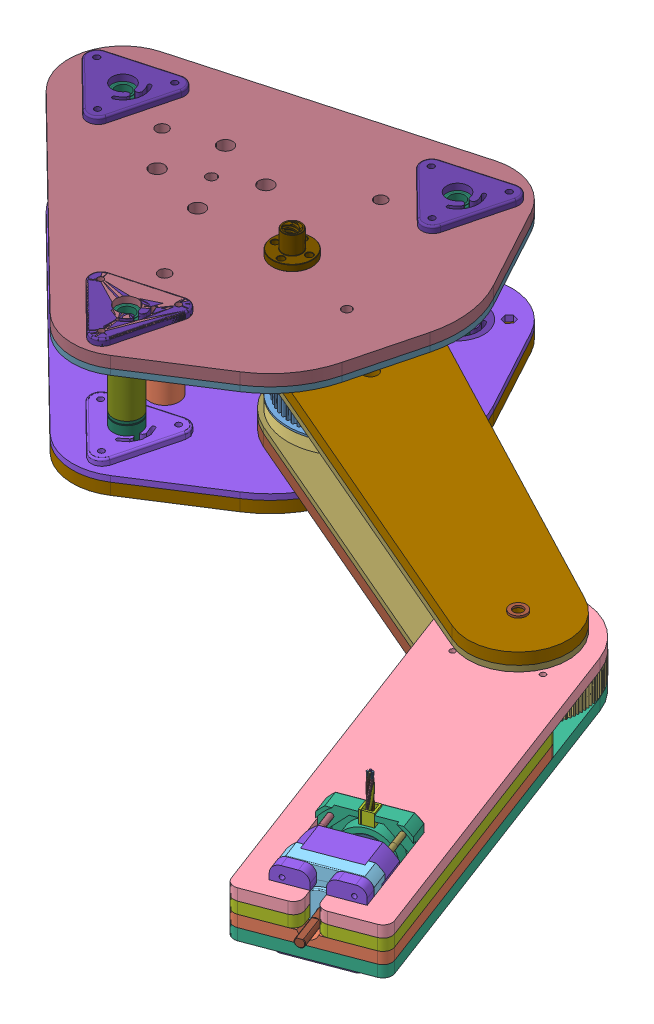
SolidWorks assembly 03_00_Assem-bras, configuration Default. Lengths in mm.
Overall size (511.83 147.28 454.98).
94 component instances, 48 part files, 15 mates.
Components (placement in the parent):
- 03_01_AssemMidArm-1: 03_01_AssemMidArm [Default] at (87.334 86.3181 -110.1057) x (0.957293 0.030604 -0.287496) z (0.28805 -0.186456 0.939288) size (98.94 97.82 258.47)
  - 7806K755_Thrust Ball Bearing-6: 7806K755_Thrust Ball Bearing [7806K755] at (-37.0592 183.6935 222.8442) x (0.999339 -0.026395 0.025015) z (-0.019643 0.187098 0.982145) size (40 14 40)
  - 7806K755_Thrust Ball Bearing-7: 7806K755_Thrust Ball Bearing [7806K755] at (-37.7539 161.4024 227.0767) x (0.408436 -0.182544 -0.894347) z (-0.912274 -0.048784 -0.406666) size (40 14 40)
  - 03_14_midArmUpper-2: 03_14_midArmUpper [Default] at (-37.5038 169.4301 225.5524) x (0.997092 -0.04302 -0.062907) z (0.069795 0.183988 0.980447) size (70 6.35 162)
  - 03_10_customPoulieDenteFinalReworkJoint1-1: 03_10_customPoulieDenteFinalReworkJoint1 [Výchozí] at (-37.4043 172.6216 224.9465) x (-0.644614 0.161957 0.747157) z (0.763896 0.097326 0.637959) size (69.97 12.55 69.97)
  - 03_14_BottomArm-2: 03_14_BottomArm [Default] at (-37.1151 181.9014 223.1844) x (0.997092 -0.04302 -0.062907) z (0.069795 0.183988 0.980447) size (70 6.35 235)
  - NEMA17 x 48.step-1: NEMA17 x 48.step [Default] at (-24.5887 206.3374 405.0196) x (0.997092 -0.04302 -0.062907) z (0.030604 0.981987 -0.186456) size (42 72 60)
    - Frontplate.step-1: Frontplate.step [Défaut] at (0 10.5 0) size (42 12.5 42)
    - Backplate.step-1: Backplate.step [Défaut] at (0 48 0) size (42 10.5 42)
    - Connenctor.step-1: Connenctor.step [Défaut] at (0 39.5 22) size (7 7 7)
    - Housing.step-1: Housing.step [Défaut] at (0 7.5 0) size (42 17 42)
    - Bearing dummy.step-1: Bearing dummy.step [Défaut] at (0 4 0) size (22 7 22)
    - Bearing dummy 01.step-1: Bearing dummy 01.step [Défaut] at (0 43 0) size (22 7 22)
    - Core.step-1: Core.step [Défaut] at origin size (30 55.5 30)
    - M3x40-Screw.step-1: M3x40-Screw.step [Default] at (15.5 45.6 15.5) x (1 0 0) z (0 1 0) size (5.5 5.5 42)
    - M3x40-Screw001.step-1: M3x40-Screw001.step [Default] at (-15.5 45.6 15.5) x (1 0 0) z (0 1 0) size (5.5 5.5 42)
    - M3x40-Screw002.step-1: M3x40-Screw002.step [Default] at (-15.5 45.6 -15.5) x (1 0 0) z (0 1 0) size (5.5 5.5 42)
    - M3x40-Screw003.step-1: M3x40-Screw003.step [Default] at (15.5 45.6 -15.5) x (1 0 0) z (0 1 0) size (5.5 5.5 42)
    - Cable-1of4.step-1: Cable-1of4.step [Défaut] at (0 43 0) size (3.44 3.69 21)
    - Copper-1of4.step-1: Copper-1of4.step [Défaut] at (0 43 0) size (2.77 3.05 24)
    - Cable-2of4.step-1: Cable-2of4.step [Défaut] at (0 43 0) x (0 1 0) z (0 0 1) size (3.44 3.69 21)
    - Copper-4of4.step-1: Copper-4of4.step [Défaut] at (0 43 0) x (0 -1 0) z (0 0 1) size (2.77 3.05 24)
    - Cable-3of4.step-1: Cable-3of4.step [Défaut] at (0 43 0) x (-1 0 0) z (0 0 1) size (3.44 3.69 21)
    - Copper-3of4.step-1: Copper-3of4.step [Défaut] at (0 43 0) x (-1 0 0) z (0 0 1) size (2.77 3.05 24)
    - Cable-4of4.step-1: Cable-4of4.step [Défaut] at (0 43 0) x (0 -1 0) z (0 0 1) size (3.44 3.69 21)
    - Copper-2of4.step-1: Copper-2of4.step [Défaut] at (0 43 0) x (0 1 0) z (0 0 1) size (2.77 3.05 24)
  - 03_13_BottomArm-3: 03_13_BottomArm [Default] at (-37.6981 163.1945 226.7364) x (0.997092 -0.04302 -0.062907) z (0.069795 0.183988 0.980447) size (70 6.35 235)
  - 03_04_midArmUpper-3: 03_04_midArmUpper [Default] at (-37.3094 175.6657 224.3684) x (0.997092 -0.04302 -0.062907) z (0.069795 0.183988 0.980447) size (70 6.35 162)
  - 03_15_SupportStepper-1: 03_15_SupportStepper [Default] at (-24.5887 206.3374 405.0196) x (0.997092 -0.04302 -0.062907) z (0.069795 0.183988 0.980447) size (57.3 42 6.35)
- 03_02_AssemUpperAndLowerArm-1: 03_02_AssemUpperAndLowerArm [Default] at (-275.5084 89.6475 14.9363) x (0.429738 0 -0.902954) z (0.902954 0 0.429738) size (70 11.12 262.5)
  - upper&lowerbearingFit3mm-1: upper&lowerbearingFit3mm [Default] at (53.4457 138.1954 313.2602) size (70 3.17 262.5) (hidden)
  - 03_07_upper&lowerArm-1: 03_07_upper&lowerArm [Default] at (53.4457 141.3704 413.2602) size (70 6.35 262.5)
  - ThrustBallBearingUpper-1: ThrustBallBearingUpper [7806K755] at (53.4457 134.3704 413.2602) x (-0.862828 0 -0.505498) z (-0.505498 0 0.862828) size (40 14 40)
- 91290A198_Black-Oxide Alloy Steel Socket Head Screw-1: 91290A198_Black-Oxide Alloy Steel Socket Head Screw [91290A198] at (120.6141 215.9679 144.2708) x (0.985537 0 -0.169459) z (0 1 0) size (8.5 8.5 55.55) (hidden)
- 98689A114_General Purpose 18-8 Stainless Steel Washer-1: 98689A114_General Purpose 18-8 Stainless Steel Washer [98689A114] at (120.6141 237.3679 144.2708) x (1 0 0) z (0 1 0) size (9 9 1.1)
- 98689A114_General Purpose 18-8 Stainless Steel Washer-2: 98689A114_General Purpose 18-8 Stainless Steel Washer [98689A114] at (120.6141 189.8678 144.2708) x (1 0 0) z (0 1 0) size (9 9 1.1)
- upper&lowerbearingFit3mm-1: upper&lowerbearingFit3mm [Default] at (30.3187 227.8429 101.2971) x (0.429738 0 -0.902954) z (0.902954 0 0.429738) size (70 3.17 262.5)
- assemblage_chariot-1: assemblage_chariot [Défaut] at (-148.1739 477.5665 143.3057) x (0.249371 0 -0.968408) z (0 -1 0) size (210 235.26 94)
  - chariot_1_4_axe_z-1: chariot_1_4_axe_z [Défaut] at (104.2914 -77.7812 228.825) size (210 232 13.03)
  - chariot_1_8_axe_z-1: chariot_1_8_axe_z [Défaut] at (104.2914 -77.7812 235.175) size (210 232 13.03)
  - LM8UU-1: LM8UU [Default] at (179.2914 22.2188 238.825) x (-0.119175 0.992873 0) z (0 0 1) size (15 15 20)
  - LM8UU-2: LM8UU [Default] at (104.2914 -107.7812 285.825) x (0.999936 0.011352 0) z (0 0 1) size (15 15 20)
  - LM8UU-3: LM8UU [Default] at (29.2914 22.2188 285.825) x (0.609724 0.792614 0) z (0 0 1) size (15 15 20)
  - LM8UU-4: LM8UU [Default] at (29.2914 22.2188 238.825) x (0.999283 -0.037866 0) z (0 0 1) size (15 15 20)
  - LM8UU-5: LM8UU [Default] at (179.2914 22.2188 285.825) size (15 15 20)
  - LM8UU-6: LM8UU [Default] at (104.2914 -107.7812 238.825) size (15 15 20)
  - spacer_bearing_chariot-1: spacer_bearing_chariot [Défaut] at (104.2914 -107.7812 248.825) x (0.653682 -0.75677 0) z (0 0 1) size (15 15 27)
  - spacer_bearing_chariot-2: spacer_bearing_chariot [Défaut] at (179.2914 22.2188 248.825) x (0.959506 -0.281688 0) z (0 0 1) size (15 15 27)
  - spacer_bearing_chariot-3: spacer_bearing_chariot [Défaut] at (29.2914 22.2188 248.825) x (0.998603 0.052836 0) z (0 0 1) size (15 15 27)
  - ancrage_bearing_lineaire-1: ancrage_bearing_lineaire [Défaut] at (179.2914 22.2188 299.325) x (-1 0 0) z (0 0 -1) size (46.22 41.63 13.03)
  - ancrage_bearing_lineaire-2: ancrage_bearing_lineaire [Défaut] at (104.2914 -107.7812 299.325) x (-1 -0.000641 0) z (0 0 -1) size (46.22 41.63 13.03)
  - ancrage_bearing_lineaire-3: ancrage_bearing_lineaire [Défaut] at (179.2914 22.2188 225.325) size (46.22 41.63 13.03)
  - ancrage_bearing_lineaire-4: ancrage_bearing_lineaire [Défaut] at (104.2914 -107.7812 225.325) x (1 0.000641 0) z (0 0 1) size (46.22 41.63 13.03)
  - ancrage_bearing_lineaire-5: ancrage_bearing_lineaire [Défaut] at (29.2914 22.2188 299.325) x (-1 -0.000641 0) z (0 0 -1) size (46.22 41.63 13.03)
  - ancrage_bearing_lineaire-6: ancrage_bearing_lineaire [Défaut] at (29.2914 22.2188 225.325) size (46.22 41.63 13.03)
  - Lead screw Nut tr8x8-4.step-1: Lead screw Nut tr8x8-4.step [Défaut] at (104.2914 22.2188 228.825) x (-0.445347 -0.895358 0) z (0 0 1) size (22 22 15)
  - Lead screw Nut tr8x8-4.step-2: Lead screw Nut tr8x8-4.step [Défaut] at (104.2914 22.2188 295.825) x (0.830203 0.557461 0) z (0 0 -1) size (22 22 15)
  - 7806K755_Thrust Ball Bearing-1: 7806K755_Thrust Ball Bearing [7806K755] at (104.2914 64.2188 242.175) x (1 0 0) z (0 -1 0) size (40 14 40)
  - 7806K755_Thrust Ball Bearing-2: 7806K755_Thrust Ball Bearing [7806K755] at (104.2914 64.2188 283.0983) x (-0.376178 0.926547 0) z (-0.926547 -0.376178 0) size (40 14 40)
  - ThrustBallBearingUpper-1: ThrustBallBearingUpper [7806K755] at (104.2914 64.2188 242.1746) x (0.97097 0.239202 0) z (-0.239202 0.97097 0) size (40 14 40)
  - ThrustBallBearingUpper-2: ThrustBallBearingUpper [7806K755] at (104.2914 64.2188 283.0986) x (0.933029 0.359801 0) z (0.359801 -0.933029 0) size (40 14 40)
  - poulie_dente_modif-1: poulie_dente_modif [Výchozí] at (104.2914 64.2188 262.6366) x (0.023795 -0.999717 0) z (-0.999717 -0.023795 0) size (65 14.22 65)
  - colonne_chariot-1: colonne_chariot [Défaut] at (153.3107 7.2188 238.35) size (16 16 48.51)
  - colonne_chariot-2: colonne_chariot [Défaut] at (55.2722 7.2188 238.35) size (16 16 48.51)
  - colonne_chariot-3: colonne_chariot [Défaut] at (104.2914 -79.7812 238.35) size (16 16 48.51)
  - appuie_1_4_poulie-1: appuie_1_4_poulie [Default] at (104.2914 64.2188 255.5246) x (0.023795 -0.999717 0) z (0.999717 0.023795 0) size (65 6.35 65)
  - appuie_1_4_poulie-2: appuie_1_4_poulie [Default] at (104.2914 64.2188 276.0986) x (-0.999717 -0.023795 0) z (0.023795 -0.999717 0) size (65 6.35 65)
  - NEMA17 x 33.step-1: NEMA17 x 33.step [Défaut] at (104.2914 -39.7812 270.7486) x (1 0 0) z (0 -1 0) size (42 57 60)
    - Copper-2of4.step-1: Copper-2of4.step [Défaut] at (0 28 0) x (0 1 0) z (0 0 1) size (2.77 3.05 24)
    - Frontplate.step-1: Frontplate.step [Défaut] at (0 10.5 0) size (42 12.5 42)
    - Backplate.step-1: Backplate.step [Défaut] at (0 33 0) size (42 10.5 42)
    - Connenctor.step-1: Connenctor.step [Défaut] at (0 24.5 22) size (7 7 7)
    - Housing.step-1: Housing.step [Défaut] at (0 7.5 0) size (42 17 42)
    - Bearing dummy.step-1: Bearing dummy.step [Défaut] at (0 4 0) size (22 7 22)
    - Bearing dummy 01.step-1: Bearing dummy 01.step [Défaut] at (0 28 0) size (22 7 22)
    - Core.step-1: Core.step [Défaut] at origin size (30 55.5 30)
    - M3x25-Screw.step-1: M3x25-Screw.step [Défaut] at (15.5 30.6 15.5) x (1 0 0) z (0 1 0) size (5.5 5.5 27)
    - M3x25-Screw004.step-1: M3x25-Screw004.step [Défaut] at (-15.5 30.6 15.5) x (1 0 0) z (0 1 0) size (5.5 5.5 27)
    - M3x25-Screw005.step-1: M3x25-Screw005.step [Défaut] at (-15.5 30.6 -15.5) x (1 0 0) z (0 1 0) size (5.5 5.5 27)
    - M3x25-Screw006.step-1: M3x25-Screw006.step [Défaut] at (15.5 30.6 -15.5) x (1 0 0) z (0 1 0) size (5.5 5.5 27)
    - Cable-1of4.step-1: Cable-1of4.step [Défaut] at (0 28 0) size (3.44 3.69 21)
    - Copper-1of4.step-1: Copper-1of4.step [Défaut] at (0 28 0) size (2.77 3.05 24)
    - Cable-2of4.step-1: Cable-2of4.step [Défaut] at (0 28 0) x (0 1 0) z (0 0 1) size (3.44 3.69 21)
    - Copper-4of4.step-1: Copper-4of4.step [Défaut] at (0 28 0) x (0 -1 0) z (0 0 1) size (2.77 3.05 24)
    - Cable-3of4.step-1: Cable-3of4.step [Défaut] at (0 28 0) x (-1 0 0) z (0 0 1) size (3.44 3.69 21)
    - Copper-3of4.step-1: Copper-3of4.step [Défaut] at (0 28 0) x (-1 0 0) z (0 0 1) size (2.77 3.05 24)
    - Cable-4of4.step-1: Cable-4of4.step [Défaut] at (0 28 0) x (0 -1 0) z (0 0 1) size (3.44 3.69 21)
  - chariot_1_8_axe_z_sans_trou_haut-2: chariot_1_8_axe_z_sans_trou_haut [Défaut] at (104.2914 -77.7812 286.3) size (210 232 13.03)
  - chariot_1_4_axe_z_sans_trou_haut-2: chariot_1_4_axe_z_sans_trou_haut [Défaut] at (104.2914 -77.7812 289.475) size (210 232 13.03)
  - support_stepper_chariot-1: support_stepper_chariot [Défaut] at (104.2914 -39.7812 235.1746) x (0 -1 0) z (0 0 1) size (42 42 35.57)
- 03_03_AssemUpperAndLowerArm_hex_tete-1: 03_03_AssemUpperAndLowerArm_hex_tete [Défaut] at (-196.1035 195.4951 -27.9706) x (0.429738 0 -0.902954) z (0.902954 0 0.429738) size (70 48.86 262.5)
  - upper&lowerbearingFit3mm-1: upper&lowerbearingFit3mm [Default] at (-19.4206 2.7978 260) size (70 3.17 262.5)
  - 03_07_upper&lowerArm_modif_tete-1: 03_07_upper&lowerArm_modif_tete [Default] at (-19.4206 -3.5522 360) size (70 6.35 262.5)
  - ThrustBallBearingUpper-1: ThrustBallBearingUpper [7806K755] at (-19.4206 9.7978 360) size (40 14 40)
Mates (geometry in assembly coordinates):
- Concentric2: concentric anti-aligned: circle of AssemMidArm-1/7806K755_Thrust Ball Bearing-6; circle of AssemUpperAndLowerArm-1/ThrustBallBearingUpper-1
- Distance1: distance = 0.5394 mm anti-aligned: plane of AssemUpperAndLowerArm-1/ThrustBallBearingUpper-1 through (137.0429 226.251 133.1122) normal (0 -1 0); plane of 03_01_AssemMidArm-1/7806K755_Thrust Ball Bearing-6 through (109.8839 225.7116 147.2647) normal (0 1 0)
- Concentric4: concentric anti-aligned: circle of AssemUpperAndLowerArm-1/upper&lowerArm-1; circle of 91290A198_Black-Oxide Alloy Steel Socket Head Screw-1
- Coincident6: coincident anti-aligned: plane of 03_02_AssemUpperAndLowerArm-1/03_07_upper&lowerArm-1 through (120.6141 237.3679 144.2708) normal (0 1 0); plane of 98689A114_General Purpose 18-8 Stainless Steel Washer-1 through (120.6141 237.3679 144.2708) normal (0 -1 0)
- Concentric6: concentric anti-aligned: circle of 91290A198_Black-Oxide Alloy Steel Socket Head Screw-1; circle of 98689A114_General Purpose 18-8 Stainless Steel Washer-1
- Coincident7: coincident anti-aligned: plane of 91290A198_Black-Oxide Alloy Steel Socket Head Screw-1 through (116.6719 238.4679 144.9487) normal (0 -1 0); plane of 98689A114_General Purpose 18-8 Stainless Steel Washer-1 through (120.6141 238.4679 144.2708) normal (0 1 0)
- Coincident9: coincident anti-aligned: plane of 90592A095_Steel Hex Nut-1 through (29.608 189.8678 96.7333) normal (0 1 0); plane of 98689A114_General Purpose 18-8 Stainless Steel Washer-2 through (120.6141 189.8678 144.2708) normal (0 -1 0)
- Coincident10: coincident anti-aligned: plane of 03_02_AssemUpperAndLowerArm-1/03_07_upper&lowerArm-1 through (120.6141 231.0179 144.2708) normal (0 -1 0); plane of upper&lowerbearingFit3mm-1 through (30.3187 231.0179 101.2971) normal (0 1 0)
- Concentric8: concentric aligned: circle of 03_01_AssemMidArm-1/03_03_midArm-3; circle of upper&lowerbearingFit3mm-1
- Coïncidente2: coincident aligned: plane of 03_01_AssemMidArm-1/03_06_customPoulieDente-1 through (120.6141 208.8179 144.2708) normal (0 1 0); plane of assemblage_chariot-1/poulie_dente_modif-1 through (-59.9767 208.8179 58.3233) normal (0 1 0)
- Coaxiale2: concentric anti-aligned: cylinder of upper&lowerbearingFit3mm-1 through (-59.9767 227.8429 58.3233) axis (0 1 0) radius 20; cylinder of assemblage_chariot-1/appuie_1_4_poulie-1 through (-59.9767 228.3919 58.3233) axis (0 -1 0) radius 32.5
- Coïncidente6: coincident aligned: plane of upper&lowerbearingFit3mm-1 through (17.9636 231.0179 129.9904) normal (-0.395485 0 0.918472); plane of 03_02_AssemUpperAndLowerArm-1/03_07_upper&lowerArm-1 through (109.7459 237.3679 169.511) normal (-0.395485 0 0.918472)
- Coïncidente7: coincident anti-aligned: plane of 03_01_AssemMidArm-1/03_03_midArm-4 through (120.6141 201.4679 144.2708) normal (0 -1 0); plane of 03_03_AssemUpperAndLowerArm_hex_tete-1/upper&lowerbearingFit3mm-1 through (30.3187 201.4679 101.2971) normal (0 1 0)
- Coaxiale3: concentric aligned: cylinder of 03_01_AssemMidArm-1/03_03_midArm-4 through (120.6141 201.4679 144.2708) axis (0 1 0) radius 21; cylinder of 03_03_AssemUpperAndLowerArm_hex_tete-1/upper&lowerbearingFit3mm-1 through (120.6141 198.2929 144.2708) axis (0 1 0) radius 20
- Coaxiale4: concentric anti-aligned: cylinder of assemblage_chariot-1/appuie_1_4_poulie-2 through (-59.9767 207.8179 58.3233) axis (0 -1 0) radius 32.5; cylinder of 03_03_AssemUpperAndLowerArm_hex_tete-1/03_07_upper&lowerArm_modif_tete-1 through (-59.9767 191.9429 58.3233) axis (0 1 0) radius 21
